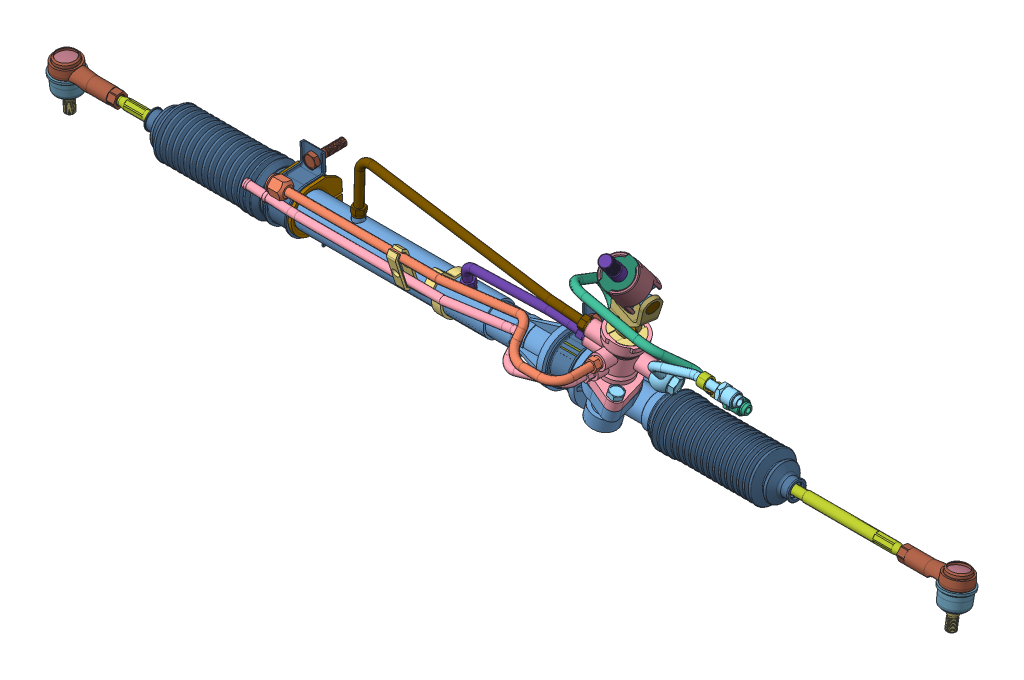
SolidWorks assembly 05, configuration Varsayılan. Lengths in mm.
Overall size (1248.7 288.74 207.21).
83 component instances, 55 part files, 117 mates.
Components (placement in the parent):
- 04-04-1: 04-04 [Varsayılan] at (-125.6681 -6.1583 231.0307) size (234.82 71.44 100.51)
- 04-02-1: 04-02 [Varsayılan] at (196.8103 -6.1583 231.0307) x (0 -1 0) z (-1 0 0) size (38 38 598)
- 04-03-1: 04-03 [Varsayılan] at (38.6923 -33.646 251.0307) x (0.503331 -0.139932 0.852688) z (-0.821509 0.228473 0.52242) size (25.52 151.51 25.52)
- 04-01-1: 04-01 [Varsayılan] at (50.1654 -6.1583 196.9106) x (0 0 1) z (-1 0 0) size (4.12 38.49 38.49)
- 04-05-1: 04-05 [Varsayılan] at (50.1654 -6.1583 220.9669) x (0 0 1) z (-1 0 0) size (15.7 26.77 26.77)
- 04-06-1: 04-06 [Varsayılan] at (50.1654 -6.1583 203.9669) x (-1 0 0) z (0 0 -1) size (18.46 18.46 19.47)
- 04-07-1: 04-07 [Varsayılan] at (50.1654 -6.1583 223.256) x (0 0 1) z (-1 0 0) size (13.68 21.45 8.13)
- 04-08-1: 04-08 [Varsayılan] at (50.1654 -6.1583 218.4607) x (0 1 0) z (-1 0 0) size (28.57 26.12 28.57)
- 05-14-1: 05-14 [Varsayılan] at (37.0194 -39.6612 251.0307) x (0.963448 -0.267897 0) z (0 0 1) size (30.59 16.59 30.59)
- 05-15-1: 05-15 [Varsayılan] at (41.4642 -23.6793 251.0307) x (0.963434 -0.267944 0) z (0 0 1) size (27.84 7.6 27.84)
- 05-21-1: 05-21 [Varsayılan] at (38.6909 -33.6508 251.0307) x (0.928206 -0.258147 -0.267944) z (0.267944 0.963434 0) size (19.84 10.08 10.35)
- 05-09-1: 05-09 [Varsayılan] at (52.7201 16.7933 251.0307) x (0.963434 -0.267944 0) z (0 0 1) size (31.93 8.54 31.93)
- 05-24-1: 05-24 [Varsayılan] at (55.0081 25.0201 251.0307) x (0.963434 -0.267944 0) z (0 0 1) size (34.48 1.46 34.48)
- 05-19-1: 05-19 [Varsayılan] at (66.8414 67.5686 251.0307) x (0.963434 -0.267944 0) z (0 0 1) size (24.62 1.21 24.62)
- 05-10-1: 05-10 [Varsayılan] at (57.7931 35.034 251.0307) x (0.959223 -0.266824 -0.093253) z (0.089843 -0.024987 0.995642) size (34.48 33.93 34.48)
- 05-11-1: 05-11 [Varsayılan] at (60.4905 44.7328 251.0307) x (0.963421 -0.267991 0) z (0 0 1) size (34.47 2.04 34.47)
- 05-11-2: 05-11 [Varsayılan] at (62.3958 51.5836 251.0307) x (0.963421 -0.267991 0) z (0 0 1) size (34.47 2.04 34.47)
- 05-11-3: 05-11 [Varsayılan] at (64.317 58.4915 251.0307) x (0.963421 -0.267991 0) z (0 0 1) size (34.47 2.04 34.47)
- 05-11-4: 05-11 [Varsayılan] at (66.1261 64.9964 251.0307) x (0.963421 -0.267991 0) z (0 0 1) size (34.47 2.04 34.47)
- 05-12-1: 05-12 [Varsayılan] at (67.6164 70.355 251.0307) x (0.92973 -0.25852 0.26224) z (-0.252651 0.070266 0.965003) size (31.17 6.94 31.17)
- 05-13-1: 05-13 [Varsayılan] at (69.4753 77.039 251.0307) x (0.963448 -0.267897 0) z (0 0 1) size (29.11 4.72 29.11)
- 05-16-1: 05-16 [Varsayılan] at (67.6164 70.3552 251.0307) x (0.963448 -0.267897 0) z (0 0 1) size (40.01 14.09 40.01)
- 05-22-3: 05-22 [Varsayılan] at (69.4711 77.024 251.0307) x (0.963434 -0.267944 0) z (0 0 1) size (37.74 2.78 37.74)
- 05-18-1: 05-18 [Varsayılan] at (71.3908 83.9266 251.0307) x (0.96127 -0.267342 0.066993) z (-0.064543 0.01795 0.997753) size (40.8 2.9 40.8)
- 05-25-1: 05-25 [Varsayılan] at (57.2884 33.5525 251.0071) x (0.003637 -0.001047 -0.999993) z (0.963428 -0.267942 0.003784) size (68.03 67.23 77.18)
- formed hex screw_am-1: formed hex screw_am [B18.2.3.2M - Formed hex screw, M10 x 1.5 x 25 --25WS] at (82.3436 33.466 275.1353) x (-0.267944 -0.963434 0) z (0 0 1) size (31.63 18.48 16)
- formed hex screw_am-2: formed hex screw_am [B18.2.3.2M - Formed hex screw, M10 x 1.5 x 25 --25WS] at (36.0727 46.3346 226.9262) x (-0.267944 -0.963434 0) z (0 0 1) size (31.63 18.48 16)
- ROT MİLİ-1: ROT MİLİ [Varsayılan] at (-410.9511 77.9473 255.0381) x (1 0 0) z (0 0.086009 -0.996294) size (284.47 41.76 37.89)
  - 02-02-2: 02-02 [Varsayılan] at (3.7615 85.8588 16.6847) size (48.52 36 36)
  - 02-03-3: 02-03 [Varsayılan] at (0.4735 85.8588 16.6847) x (-1 0 0) z (0 0.000479 1) size (257.66 24 24)
  - 02-01-2: 02-01 [Varsayılan] at (2.815 90.0301 15.9062) x (0.295289 -0.871295 0.391981) z (-0.068342 0.389963 0.918291) size (28 21.64 28)
- ROT MİLİ-2: ROT MİLİ [Varsayılan] at (206.5718 -67.283 293.5918) x (-1 0 0) z (0 -0.568825 -0.822459) size (284.47 41.76 37.89)
  - 02-02-2: 02-02 [Varsayılan] at (3.7615 85.8588 16.6847) size (48.52 36 36)
  - 02-03-3: 02-03 [Varsayılan] at (0.4735 85.8588 16.6847) x (-1 0 0) z (0 0.000479 1) size (257.66 24 24)
  - 02-01-2: 02-01 [Varsayılan] at (2.815 90.0301 15.9062) x (0.295289 -0.871295 0.391981) z (-0.068342 0.389963 0.918291) size (28 21.64 28)
- 05-31-1: 05-31 [Varsayılan] at (-390.0863 -6.1583 231.0307) x (0 0.999978 0.006566) z (0 0.006566 -0.999978) size (59.07 38.45 68.81)
- 05-02-1: 05-02 [Varsayılan] at (-409.0863 -6.1583 231.0307) x (-1 0 0) z (0 -0.999688 0.024965) size (174.75 66.11 66.11)
- 05-02-2: 05-02 [Varsayılan] at (105.6183 -6.1583 231.0307) size (174.75 66.11 66.11)
- ROT BAŞI-1: ROT BAŞI [Varsayılan] at (-661.705 -10.787 321.1728) x (1 0 0) z (0 0.078367 -0.996925) size (99.29 68.51 54.56)
  - 03-01-1: 03-01 [Default] at (-37.7726 9.1069 90.2276) size (90.23 26.88 54.56)
  - 03-02-1: 03-02 [Varsayılan] at (-32.6694 53.6205 89.5242) x (0 -1 0) z (0.136534 0 0.990635) size (58.89 20 20)
  - 03-03-1: 03-03 [Varsayılan] at (-37.7726 -12.3176 90.2276) x (0.135044 0.003215 -0.990834) z (0.99084 0 0.135044) size (26.35 4.4 26.35)
  - 03-04-1: 03-04 [Varsayılan] at (-37.7726 28.686 90.2276) x (0.880691 0 -0.473691) z (0.473691 0 0.880691) size (39.96 25.57 39.96)
  - 03-05-1: 03-05 [Varsayılan] at (-37.7726 -9.866 90.2276) size (25.83 14.98 25.83)
- ROT BAŞI-2: ROT BAŞI [Varsayılan] at (457.3257 -18.6564 141.6394) x (-1 0 0) z (0 0.1653 0.986243) size (99.29 68.51 54.56)
  - 03-01-1: 03-01 [Default] at (-37.7726 9.1069 90.2276) size (90.23 26.88 54.56)
  - 03-02-1: 03-02 [Varsayılan] at (-32.6694 53.6205 89.5242) x (0 -1 0) z (0.136534 0 0.990635) size (58.89 20 20)
  - 03-03-1: 03-03 [Varsayılan] at (-37.7726 -12.3176 90.2276) x (0.135044 0.003215 -0.990834) z (0.99084 0 0.135044) size (26.35 4.4 26.35)
  - 03-04-1: 03-04 [Varsayılan] at (-37.7726 28.686 90.2276) x (0.880691 0 -0.473691) z (0.473691 0 0.880691) size (39.96 25.57 39.96)
  - 03-05-1: 03-05 [Varsayılan] at (-37.7726 -9.866 90.2276) size (25.83 14.98 25.83)
- 05-28-1: 05-28 [Varsayılan] at (-1.0263 -6.1583 231.0307) x (0 -0.759317 -0.650721) z (-1 0 0) size (54.92 54.94 38.56)
- 05-05-3: 05-05 [Varsayılan] at (-153.627 16.7021 236.5228) x (-0.999618 0.007048 -0.026719) z (0.027616 0.221471 -0.974776) size (188.63 111.65 20.5)
- 05-06-2: 05-06 [Varsayılan] at (-308.371 55.2453 229.576) x (-0.999565 0.002273 -0.029406) z (0.029339 -0.025305 -0.999249) size (348.36 140.05 41.18)
- 05-03-3: 05-03 [Varsayılan] at (-414.0863 -6.1583 231.0307) size (295 48.35 43.5)
- 05-33-1: 05-33 [Default] at (-156.8797 44.8002 297.1129) x (-1 0 0) z (0 0.302472 -0.953158) size (421.56 52.06 61.28)
- 05-01-1: 05-01 [Varsayılan] at (-173.5526 -6.1583 231.0307) x (-1 0 0) z (0 0.360562 -0.932735) size (14 137.7 76.92)
- 05-04-1: 05-04 [Varsayılan] at (-390.9146 51.2479 300.523) x (-0.991921 0.112405 0.058801) z (0.000453 0.46666 -0.884437) size (456.96 84.72 60.32)
- 05-08-1: 05-08 [Varsayılan] at (237.637 92.2948 265.4276) x (-0.997325 0.072053 -0.012308) z (-0.043043 -0.714977 -0.697822) size (140.05 46.48 89.04)
- 05-07-1: 05-07 [Varsayılan] at (228.5019 70.3353 246.6946) x (-0.999175 0.040461 0.003581) z (-0.026401 -0.579908 -0.814254) size (231 45.96 100.61)
- formed hex screw_am-3: formed hex screw_am [B18.2.3.2M - Formed hex screw, M12 x 1.75 x 25 --25WS] at (123.6594 37.5337 232.8376) x (-0.948079 0.263674 0.177825) z (-0.177825 -0.903067 0.390959) size (32.76 20.78 18)
- 05-27-1: 05-27 [Varsayılan] at (186.4406 76.9952 250.3773) x (0.044464 0.751851 0.657832) z (0.9987 -0.049876 -0.0105) size (45.68 8 10)
- 05-27-2: 05-27 [Varsayılan] at (196.4276 76.4964 250.2723) x (0.044464 0.751851 0.657832) z (-0.9987 0.049876 0.0105) size (45.68 8 10)
- hex screw_am-2: hex screw_am [B18.6.7M - M5 x 0.8 x 10 Indented HHMS --10S] at (191.9929 87.5632 252.0852) x (-0.024915 -0.657444 0.753091) z (-0.753091 0.507767 0.418362) size (13.8 9.24 8)
- prevailing torque hex nut_am-2: prevailing torque hex nut_am [AM-M5-S] at (191.6665 78.9507 261.9507) x (0.999646 -0.009344 0.024915) z (-0.024915 -0.657444 0.753091) size (8 9.24 5.3)
- 05-29-1: 05-29 [Default] at (-12.3188 -6.1583 205.6444) x (0 1 0) z (0 0 -1) size (108.96 30.28 55.85)
- 05-29-3: 05-29 [Default] at (-390.1285 -6.1115 206.1523) x (0 0.999914 0.013132) z (0 0.013132 -0.999914) size (108.96 30.28 55.85)
- 05-32-2: 05-32 [B18.2.3.2M - Formed hex screw, M10 x 1.5 x 40 --26WS] at (-390.1268 33.0747 215.2976) x (0 0.013132 -0.999914) z (0.935126 0.354284 0.004653) size (46.63 18.48 16)
- 05-32-3: 05-32 [B18.2.3.2M - Formed hex screw, M10 x 1.5 x 40 --26WS] at (-390.1268 -45.812 214.2616) x (0 0.013132 -0.999914) z (0.970956 -0.239236 -0.003142) size (46.63 18.48 16)
- 05-32-4: 05-32 [B18.2.3.2M - Formed hex screw, M10 x 1.5 x 40 --26WS] at (-12.3171 -45.7489 214.2744) x (0 0 -1) z (0.991782 -0.12794 0) size (46.63 18.48 16)
- 05-32-5: 05-32 [B18.2.3.2M - Formed hex screw, M10 x 1.5 x 40 --26WS] at (-12.3171 33.1445 213.7744) x (0 0 -1) z (0.999706 0.024251 0) size (46.63 18.48 16)
- UNIVERSAL MAFSAL-1: UNIVERSAL MAFSAL [Varsayılan] at (141.1705 165.1329 255.0986) x (0.954818 -0.265548 0.133442) z (-0.267944 -0.963434 0) size (48.16 92.97 129.43)
  - 01-01-1: 01-01 [Varsayılan] at (-45.6055 2.036 86.4549) size (47 34.99 57.64)
  - 01-02-1: 01-02 [Varsayılan] at (-45.0363 8.2494 31.8587) x (-0.051046 -0.624854 0.779071) z (0 -0.780088 -0.62567) size (70.3 43.23 43.34)
  - 01-03-1: 01-03 [Varsayılan] at (-51.6055 -0.2661 32.8861) x (1 0 0) z (0 -0.62567 0.780088) size (36 31 16)
  - 01-04-1: 01-04 [Varsayılan] at (-42.5986 38.09 -5.3467) x (-0.998696 0.031938 -0.03982) z (-0.051046 -0.624854 0.779071) size (33.8 41.3 6)
  - 01-05-1: 01-05 [Varsayılan] at (-42.9049 34.3409 -0.6723) x (0.998255 -0.008733 0.058403) z (0.02969 -0.780692 -0.62421) size (32.2 29.4 32.2)
  - 01-06-1: 01-06 [Varsayılan] at (-44.4056 15.9701 22.2324) x (0.051046 0.624854 -0.779071) z (0.993628 0.046715 0.102572) size (75.7 17.29 17.32)
  - 01-07-1: 01-07 [Varsayılan] at (-25.3055 1.2861 40.5406) x (0 0 -1) z (1 0 0) size (16 16 15)
  - 01-08-1: 01-08 [Varsayılan] at (-45.6055 -12.5995 29.4036) x (0.792707 0.38141 -0.475544) z (0 -0.780088 -0.62567) size (16 16 15)
  - 01-07-2: 01-07 [Varsayılan] at (-65.9055 1.2861 40.5406) x (0 -0.633294 0.773912) z (-1 0 0) size (16 16 15)
  - 01-08-2: 01-08 [Varsayılan] at (-45.6055 15.1716 51.6775) x (0.990366 0.086641 -0.108024) z (0 0.780088 0.62567) size (16 16 15)
  - formed hex screw_am-1: formed hex screw_am [B18.2.3.2M - Formed hex screw, M6 x 1.0 x 35 --18WS] at (-62.5055 12.536 76.9549) x (1 0 0) z (0 0.052048 -0.998645) size (39.15 11.55 10)
  - prevailing torque hex nut_am-1: prevailing torque hex nut_am [AM-M6-S] at (-26.1555 12.536 76.9549) x (0 0.889289 0.457347) z (1 0 0) size (10.79 11.55 6.7)
Mates (geometry in assembly coordinates):
- Eş Merkezli1: concentric aligned: cylinder of 04-04-1 through (-165.266 -6.1583 231.0307) axis (1 0 0) radius 14; cylinder of 04-02-1 through (-401.1897 -6.1583 231.0307) axis (1 0 0) radius 11.5
- Eş Merkezli2: concentric anti-aligned: cylinder of 04-04-1 through (54.1024 21.7633 251.0307) axis (0.267944 0.963434 0) radius 12.4576; line of 04-03-1 through (79.2895 112.3276 251.0307) axis (-0.267944 -0.963434 0)
- Teğet1: tangent aligned: plane of 04-04-1 through (55.5026 -19.6951 251.0307) normal (-0.267944 -0.963434 0); cone of 04-03-1 through (43.5006 -16.357 251.0307) axis (-0.267944 -0.963434 0)
- Paralel1: parallel: plane of 04-02-1 through (33.8834 10.9835 238.0307) normal (0 0 1); line of 04-03-1 through (79.2895 112.3276 251.0307) axis (-0.267944 -0.963434 0)
- RackPinionMate1: rack pinion = 20 mm: line of 04-02-1 through (-6.8954 -15.2825 238.0307) axis (-1 0 0); circle of 04-03-1
- Uzaklığı Sınırla1: limit distance = 59.5855 mm anti-aligned: plane of 04-04-1 through (-125.6681 11.3406 231.0307) normal (-1 0 0); plane of 04-02-1 through (-183.1897 -6.1583 250.0307) normal (1 0 0)
- Eş Merkezli3: concentric anti-aligned: cylinder of 04-05-1 through (50.1654 -6.1583 220.9669) axis (0 0 -1) radius 3.705; cylinder of 04-07-1 through (50.1654 -6.1583 223.256) axis (0 0 1) radius 3.7071
- Eş Merkezli4: concentric: sphere of 04-05-1; sphere of 04-07-1
- Eş Merkezli5: concentric anti-aligned: circle of 04-06-1; cylinder of 04-07-1 through (50.1654 -6.1583 223.256) axis (0 0 1) radius 3.7071
- Çakışık1: coincident anti-aligned: plane of 04-05-1 through (59.8031 -6.1583 220.9669) normal (0 0 -1); plane of 04-06-1 through (40.4527 -15.387 220.9669) normal (0 0 1)
- Eş Merkezli6: concentric anti-aligned: circle of 04-06-1; cylinder of 04-08-1 through (50.1654 -6.1583 199.3607) axis (0 0 1) radius 14.285
- Çakışık2: coincident anti-aligned: plane of 04-05-1 through (63.3694 -6.1583 218.4607) normal (0 0 -1); plane of 04-08-1 through (50.1654 -6.1583 218.4607) normal (0 0 1)
- Eş Merkezli7: concentric anti-aligned: cylinder of 04-04-1 through (50.1654 -6.1583 285.0814) axis (0 0 -1) radius 14; cylinder of 04-08-1 through (50.1654 -6.1583 199.3607) axis (0 0 1) radius 14.285
- Çakışık3: coincident anti-aligned: plane of 04-04-1 through (50.1654 -6.1583 201.0307) normal (0 0 -1); circle of 04-08-1
- Eş Merkezli8: concentric anti-aligned: cylinder of 04-04-1 through (50.1654 -6.1583 201.0307) axis (0 0 1) radius 18.85; cylinder of 04-01-1 through (50.1654 -6.1583 196.9106) axis (0 0 -1) radius 13.3852
- Çakışık4: coincident anti-aligned: plane of 04-04-1 through (50.1654 -6.1583 201.0307) normal (0 0 -1); plane of 04-01-1 through (63.5506 -6.1583 201.0307) normal (0 0 1)
- Eş Merkezli9: concentric anti-aligned: cylinder of 04-04-1 through (54.1024 21.7633 251.0307) axis (0.267944 0.963434 0) radius 15.0252; cylinder of 05-15-1 through (43.5005 -16.3572 251.0307) axis (-0.267944 -0.963434 0) radius 13.92
- Çakışık5: coincident anti-aligned: plane of 04-04-1 through (55.5026 -19.6951 251.0307) normal (-0.267944 -0.963434 0); plane of 05-15-1 through (43.5005 -16.3572 251.0307) normal (0.267944 0.963434 0)
- Eş Merkezli10: concentric aligned: cone of 04-03-1 through (38.6923 -33.6458 251.0307) axis (0.267944 0.963434 0); cylinder of 05-21-1 through (38.6909 -33.6508 251.0307) axis (0.267944 0.963434 0) radius 4.26
- Çakışık6: coincident anti-aligned: plane of 05-15-1 through (41.4642 -23.6793 251.0307) normal (-0.267944 -0.963434 0); plane of 05-21-1 through (41.4642 -23.6793 251.0307) normal (0.267944 0.963434 0)
- Eş Merkezli11: concentric aligned: cylinder of 04-04-1 through (54.1024 21.7633 251.0307) axis (0.267944 0.963434 0) radius 15.0252; cone of 05-14-1 through (39.1828 -31.8821 251.0307) axis (0.267944 0.963434 0)
- Teğet2: tangent aligned: cone of 05-14-1 through (41.4644 -23.6786 251.0307) axis (-0.267944 -0.963434 0); plane of 05-15-1 through (41.4642 -23.6793 251.0307) normal (-0.267944 -0.963434 0)
- Çakışık7: coincident: circle of 04-03-1; cone of 05-09-1 through (52.7203 16.7939 251.0307) axis (-0.267944 -0.963434 0)
- Eş Merkezli13: concentric anti-aligned: cylinder of 04-03-1 through (38.6923 -33.646 251.0307) axis (-0.267944 -0.963434 0) radius 12.7592; cone of 05-24-1 through (55.3985 26.4236 251.0307) axis (0.267944 0.963434 0)
- Çakışık8: coincident aligned: cone of 05-09-1 through (55.0081 25.0199 251.0307) axis (-0.267944 -0.963434 0); cone of 05-24-1 through (55.0081 25.0201 251.0307) axis (-0.267944 -0.963434 0)
- Eş Merkezli14: concentric anti-aligned: cone of 04-03-1 through (67.1664 68.7371 251.0307) axis (0.267944 0.963434 0); circle of 05-19-1
- Teğet4: tangent aligned: cone of 04-03-1 through (66.8416 67.5691 251.0307) axis (-0.267944 -0.963434 0); plane of 05-19-1 through (66.8414 67.5686 251.0307) normal (-0.267944 -0.963434 0)
- Eş Merkezli15: concentric anti-aligned: cone of 04-03-1 through (67.1664 68.7371 251.0307) axis (0.267944 0.963434 0); cone of 05-10-1 through (58.0415 35.927 251.0307) axis (-0.267944 -0.963434 0)
- Teğet5: tangent aligned: plane of 05-19-1 through (66.8414 67.5686 251.0307) normal (-0.267944 -0.963434 0); cone of 05-10-1 through (66.8416 67.5691 251.0307) axis (-0.267944 -0.963434 0)
- Eş Merkezli17: concentric aligned: cone of 05-10-1 through (60.4905 44.7328 251.0307) axis (0.267944 0.963434 0); cone of 05-11-1 through (61.036 46.6944 251.0307) axis (0.267944 0.963434 0)
- Çakışık10: coincident: circle of 05-10-1; cone of 05-11-1 through (60.4905 44.7328 251.0307) axis (-0.267944 -0.963434 0)
- Eş Merkezli18: concentric aligned: cone of 05-10-1 through (62.3958 51.5836 251.0307) axis (0.267944 0.963434 0); cone of 05-11-2 through (62.9414 53.5453 251.0307) axis (0.267944 0.963434 0)
- Çakışık11: coincident: circle of 05-10-1; cone of 05-11-2 through (62.3958 51.5836 251.0307) axis (-0.267944 -0.963434 0)
- Eş Merkezli19: concentric aligned: cone of 05-10-1 through (64.317 58.4915 251.0307) axis (0.267944 0.963434 0); cone of 05-11-3 through (64.8625 60.4532 251.0307) axis (0.267944 0.963434 0)
- Çakışık12: coincident: circle of 05-10-1; cone of 05-11-3 through (64.317 58.4915 251.0307) axis (-0.267944 -0.963434 0)
- Eş Merkezli20: concentric aligned: cone of 05-10-1 through (66.1261 64.9964 251.0307) axis (0.267944 0.963434 0); cone of 05-11-4 through (66.6716 66.958 251.0307) axis (0.267944 0.963434 0)
- Çakışık13: coincident: circle of 05-10-1; cone of 05-11-4 through (66.1261 64.9964 251.0307) axis (-0.267944 -0.963434 0)
- Eş Merkezli22: concentric aligned: cone of 04-03-1 through (67.1664 68.7371 251.0307) axis (0.267944 0.963434 0); cone of 05-12-1 through (69.4753 77.039 251.0307) axis (0.267944 0.963434 0)
- Uzaklık1: distance = 2.73 mm aligned: cone of 05-12-1 through (67.6164 70.355 251.0307) axis (-0.267944 -0.963434 0); cone of 05-10-1 through (66.885 67.7251 251.0307) axis (-0.267944 -0.963434 0)
- Eş Merkezli23: concentric aligned: cone of 04-03-1 through (67.1664 68.7371 251.0307) axis (0.267944 0.963434 0); cone of 05-13-1 through (70.7393 81.584 251.0307) axis (0.267944 0.963434 0)
- Çakışık14: coincident aligned: cone of 05-12-1 through (69.4754 77.0393 251.0307) axis (-0.267944 -0.963434 0); cone of 05-13-1 through (69.4753 77.039 251.0307) axis (-0.267944 -0.963434 0)
- Eş Merkezli24: concentric aligned: cone of 05-12-1 through (67.6164 70.3552 251.0307) axis (0.267944 0.963434 0); cone of 05-16-1 through (67.6165 70.3554 251.0307) axis (0.267944 0.963434 0)
- Çakışık15: coincident aligned: cone of 05-12-1 through (67.6164 70.355 251.0307) axis (-0.267944 -0.963434 0); cone of 05-16-1 through (67.6164 70.3552 251.0307) axis (-0.267944 -0.963434 0)
- Eş Merkezli25: concentric anti-aligned: cone of 05-16-1 through (69.4711 77.024 251.0307) axis (0.267944 0.963434 0); cylinder of 05-22-3 through (70.216 79.7023 251.0307) axis (-0.267944 -0.963434 0) radius 18.87
- Çakışık16: coincident aligned: circle of 05-16-1; plane of 05-22-3 through (69.4711 77.024 251.0307) normal (-0.267944 -0.963434 0)
- Eş Merkezli26: concentric anti-aligned: cone of 04-03-1 through (67.1664 68.7371 251.0307) axis (0.267944 0.963434 0); cylinder of 05-18-1 through (76.455 102.1355 251.0307) axis (-0.267944 -0.963434 0) radius 9.8
- Teğet6: tangent aligned: cone of 05-16-1 through (71.3911 83.9275 251.0307) axis (-0.267944 -0.963434 0); plane of 05-18-1 through (71.3908 83.9266 251.0307) normal (-0.267944 -0.963434 0)
- Eş Merkezli27: concentric aligned: cylinder of 04-04-1 through (47.6487 -91.2848 275.1353) axis (0.267944 0.963434 0) radius 5.0797; cylinder of 05-25-1 through (77.2955 15.3149 275.1353) axis (0.267944 0.963434 0) radius 4.95
- Eş Merkezli28: concentric aligned: cylinder of 04-04-1 through (1.3778 -78.4162 226.9262) axis (0.267944 0.963434 0) radius 4.95; cylinder of 05-25-1 through (31.0246 28.1834 226.9262) axis (0.267944 0.963434 0) radius 5.0797
- Çakışık17: coincident anti-aligned: plane of 04-04-1 through (81.3463 14.1883 251.0307) normal (0.267944 0.963434 0); plane of 05-25-1 through (54.0168 21.789 251.0071) normal (-0.267944 -0.963434 0)
- Eş Merkezli291: concentric aligned: cylinder of 05-25-1 through (77.2955 15.3149 275.1353) axis (0.267944 0.963434 0) radius 4.95; cylinder of formed hex screw_am-1 through (82.3436 33.466 275.1353) axis (0.267944 0.963434 0) radius 5
- Çakışık181: coincident anti-aligned: plane of 05-25-1 through (57.2884 33.5525 251.0071) normal (0.267944 0.963434 0); plane of formed hex screw_am-1 through (89.4669 24.6032 275.1353) normal (-0.267944 -0.963434 0)
- Eş Merkezli301: concentric aligned: cylinder of 05-25-1 through (31.0246 28.1834 226.9262) axis (0.267944 0.963434 0) radius 5.0797; cylinder of formed hex screw_am-2 through (36.0727 46.3346 226.9262) axis (0.267944 0.963434 0) radius 5
- Çakışık191: coincident anti-aligned: plane of 05-25-1 through (57.2884 33.5525 251.0071) normal (0.267944 0.963434 0); plane of formed hex screw_am-2 through (43.196 37.4718 226.9262) normal (-0.267944 -0.963434 0)
- Eş Merkezli32: concentric anti-aligned: cylinder of 04-02-1 through (-401.1897 -6.1583 231.0307) axis (1 0 0) radius 11.5; cylinder of ROT MİLİ-1/02-02-2 through (-407.3432 -6.1583 231.0307) axis (-1 0 0) radius 18
- Çakışık20: coincident anti-aligned: plane of 04-02-1 through (-401.1897 -6.1583 231.0307) normal (-1 0 0); plane of ROT MİLİ-1/02-02-2 through (-401.1897 -6.1583 231.0307) normal (1 0 0)
- Eş Merkezli33: concentric aligned: cylinder of 04-02-1 through (-401.1897 -6.1583 231.0307) axis (1 0 0) radius 11.5; cylinder of ROT MİLİ-2/02-02-2 through (202.9638 -6.1583 231.0307) axis (1 0 0) radius 18
- Çakışık21: coincident anti-aligned: plane of 04-02-1 through (196.8103 -6.1583 231.0307) normal (1 0 0); plane of ROT MİLİ-2/02-02-2 through (196.8103 -6.1583 231.0307) normal (-1 0 0)
- Eş Merkezli36: concentric anti-aligned: cylinder of 04-02-1 through (-401.1897 -6.1583 231.0307) axis (1 0 0) radius 11.5; cylinder of 05-02-2 through (105.6183 -6.1583 231.0307) axis (-1 0 0) radius 11.6806
- Çakışık23: coincident anti-aligned: plane of 04-04-1 through (105.6183 12.6764 231.0307) normal (1 0 0); plane of 05-02-2 through (105.6183 19.7754 231.0307) normal (-1 0 0)
- Eş Merkezli37: concentric aligned: cylinder of ROT MİLİ-1/02-03-3 through (-421.4776 -6.1583 231.0307) axis (1 0 0) radius 5.0675; cylinder of ROT BAŞI-1/03-01-1 through (-664.2276 -6.1583 231.0307) axis (1 0 0) radius 9.5
- Çakışık24: coincident aligned: circle of ROT MİLİ-1/02-03-3; plane of ROT BAŞI-1/03-01-1 through (-627.4776 3.069 222.1124) normal (1 0 0)
- Eş Merkezli38: concentric aligned: cylinder of ROT MİLİ-2/02-03-3 through (217.0983 -6.1583 231.0307) axis (-1 0 0) radius 6.5; cylinder of ROT BAŞI-2/03-01-1 through (459.8483 -6.1579 231.0307) axis (-1 0 0) radius 9.5
- Çakışık25: coincident aligned: circle of ROT MİLİ-2/02-03-3; plane of ROT BAŞI-2/03-01-1 through (423.0983 3.8144 239.1074) normal (-1 0 0)
- Eş Merkezli39: concentric anti-aligned: cylinder of 04-04-1 through (-125.6681 -6.1583 231.0307) axis (-1 0 0) radius 21.75; cylinder of 05-28-1 through (-23.5863 -6.1583 231.0307) axis (1 0 0) radius 25.75
- Çakışık26: coincident anti-aligned: plane of 04-04-1 through (6.9737 26.3417 231.0307) normal (-1 0 0); plane of 05-28-1 through (6.9737 -6.1583 231.0307) normal (1 0 0)
- Eş Merkezli304: concentric anti-aligned: cylinder of 05-25-1 through (101.3768 36.6462 241.4658) axis (-0.949417 0.264046 0.169963) radius 5; cylinder of 05-05-3 through (21.6687 58.8141 255.7351) axis (0.949417 -0.264046 -0.169963) radius 7
- Çakışık194: coincident anti-aligned: plane of 05-25-1 through (21.5918 48.3269 253.9468) normal (-0.949417 0.264046 0.169963); plane of 05-05-3 through (26.0012 62.678 256.2827) normal (0.949417 -0.264046 -0.169963)
- Eş Merkezli305: concentric anti-aligned: cylinder of 05-25-1 through (105.7565 50.9201 243.7559) axis (-0.949417 0.264046 0.169963) radius 5; cylinder of 05-06-2 through (26.0484 73.088 258.0251) axis (0.949417 -0.264046 -0.169963) radius 7
- Çakışık195: coincident anti-aligned: plane of 05-25-1 through (21.5918 48.3269 253.9468) normal (-0.949417 0.264046 0.169963); plane of 05-06-2 through (30.1982 77.1184 257.2936) normal (0.949417 -0.264046 -0.169963)
- Eş Merkezli306: concentric anti-aligned: cylinder of 04-02-1 through (-401.1897 -6.1583 231.0307) axis (1 0 0) radius 11.5; cylinder of 05-03-3 through (-119.0863 -6.1583 231.0307) axis (-1 0 0) radius 21.75
- Çakışık196: coincident anti-aligned: plane of 04-04-1 through (-119.0863 12.8417 231.0307) normal (-1 0 0); plane of 05-03-3 through (-119.0863 -6.1583 231.0307) normal (1 0 0)
- Eş Merkezli307: concentric anti-aligned: cylinder of 05-31-1 through (-405.0863 -6.1583 231.0307) axis (1 0 0) radius 20.7084; cylinder of 05-03-3 through (-119.0863 -6.1583 231.0307) axis (-1 0 0) radius 21.75
- Eş Merkezli308: concentric anti-aligned: cylinder of 05-02-1 through (-409.0863 -6.1583 231.0307) axis (1 0 0) radius 25.6827; cylinder of 05-03-3 through (-119.0863 -6.1583 231.0307) axis (-1 0 0) radius 21.75
- Uzaklık2: distance = 5 mm aligned: plane of 05-03-3 through (-414.0863 -6.1583 231.0307) normal (-1 0 0); plane of 05-31-1 through (-409.0863 -6.1583 231.0307) normal (-1 0 0)
- Çakışık197: coincident anti-aligned: plane of 05-31-1 through (-409.0863 -6.1583 231.0307) normal (-1 0 0); plane of 05-02-1 through (-409.0863 -6.8058 205.105) normal (1 0 0)
- Kilitle1: lock: unknown of 05-05-3; unknown of 05-03-3
- Kilitle2: lock: unknown of 05-06-2; unknown of 05-03-3
- Eş Merkezli309: concentric anti-aligned: cylinder of 05-25-1 through (65.5394 62.2675 263.2963) axis (-0.003655 0.006527 0.999972) radius 5; cylinder of 05-33-1 through (65.3201 62.6591 323.2946) axis (0.003655 -0.006527 -0.999972) radius 4
- Çakışık198: coincident anti-aligned: plane of 05-25-1 through (60.6154 54.5186 283.3295) normal (-0.003655 0.006527 0.999972); plane of 05-33-1 through (65.4663 62.3981 283.2958) normal (0.003655 -0.006527 -0.999972)
- Eş Merkezli310: concentric anti-aligned: cylinder of 05-03-3 through (-119.0863 -6.1583 231.0307) axis (-1 0 0) radius 21.75; cylinder of 05-01-1 through (-185.5526 -6.1583 231.0307) axis (1 0 0) radius 21.7671
- Teğet7: tangent anti-aligned: cylinder of 05-33-1 through (-125.1716 75.9211 306.9887) axis (-1 0 0) radius 5; plane of 05-01-1 through (-172.5526 79.1244 302.774) normal (0 -0.309917 0.950763)
- Eş Merkezli312: concentric anti-aligned: cylinder of 05-25-1 through (55.8376 46.5086 263.3637) axis (-0.003655 0.006527 0.999972) radius 5; circle of 05-04-1
- Çakışık201: coincident anti-aligned: plane of 05-25-1 through (60.6154 54.5186 283.3295) normal (-0.003655 0.006527 0.999972); plane of 05-04-1 through (60.0822 49.1995 283.3622) normal (0.003655 -0.006527 -0.999972)
- Kilitle3: lock: unknown of 05-01-1; unknown of 05-04-1
- Eş Merkezli313: concentric aligned: cylinder of 05-25-1 through (18.9204 66.663 252.4828) axis (0.948079 -0.263674 -0.177825) radius 5; cylinder of 05-08-1 through (83.9328 48.5821 240.2888) axis (0.948079 -0.263674 -0.177825) radius 5
- Çakışık202: coincident anti-aligned: plane of 05-25-1 through (97.3407 44.8532 237.774) normal (0.948079 -0.263674 -0.177825); plane of 05-08-1 through (101.3663 42.9237 262.0976) normal (-0.948079 0.263674 0.177825)
- Eş Merkezli314: concentric anti-aligned: cylinder of 05-25-1 through (91.8203 46.3885 292.2446) axis (-0.66663 0.185399 -0.721963) radius 5; cylinder of 05-07-1 through (28.8333 63.9061 224.0295) axis (0.66663 -0.185399 0.721963) radius 3
- Çakışık203: coincident anti-aligned: plane of 05-25-1 through (40.3095 60.7144 222.006) normal (-0.66663 0.185399 -0.721963); plane of 05-07-1 through (29.8159 63.3842 232.381) normal (0.66663 -0.185399 0.721963)
- Eş Merkezli3151: concentric aligned: cylinder of 05-08-1 through (83.9328 48.5821 240.2888) axis (0.948079 -0.263674 -0.177825) radius 5; cylinder of formed hex screw_am-3 through (123.6594 37.5337 232.8376) axis (0.948079 -0.263674 -0.177825) radius 6
- Çakışık2041: coincident anti-aligned: plane of 05-08-1 through (120.4882 37.9933 258.8874) normal (0.948079 -0.263674 -0.177825); plane of formed hex screw_am-3 through (113.5621 36.0564 224.8326) normal (-0.948079 0.263674 0.177825)
- Eş Merkezli316: concentric anti-aligned: cylinder of 05-08-1 through (180.9639 95.1251 266.0234) axis (0.9987 -0.049876 -0.0105) radius 5; cylinder of 05-27-1 through (197.4805 94.3003 265.8497) axis (-0.9987 0.049876 0.0105) radius 8
- Kilitle4: lock: unknown of 05-07-1; unknown of 05-27-1
- Eş Merkezli320: concentric anti-aligned: cylinder of 05-27-1 through (191.5494 75.8607 265.4902) axis (0.024915 0.657444 -0.753091) radius 2.5; cylinder of 05-27-2 through (192.1473 91.6394 247.416) axis (-0.024915 -0.657444 0.753091) radius 2.5
- Çakışık206: coincident anti-aligned: plane of 05-27-1 through (196.4276 76.4964 250.2723) normal (0.024915 0.657444 -0.753091); plane of 05-27-2 through (186.4406 76.9952 250.3773) normal (-0.024915 -0.657444 0.753091)
- Paralel2: parallel aligned: plane of 05-27-1 through (196.1608 71.9853 246.3253) normal (0.9987 -0.049876 -0.0105); plane of 05-27-2 through (196.1608 71.9853 246.3253) normal (0.9987 -0.049876 -0.0105)
- Eş Merkezli3221: concentric anti-aligned: cylinder of 05-27-2 through (192.1473 91.6394 247.416) axis (-0.024915 -0.657444 0.753091) radius 2.5; cylinder of hex screw_am-2 through (192.6257 104.2623 232.9567) axis (0.024915 0.657444 -0.753091) radius 2.5
- Çakışık2091: coincident anti-aligned: plane of 05-27-2 through (187.1989 90.2901 259.353) normal (0.024915 0.657444 -0.753091); plane of hex screw_am-2 through (193.5418 86.4567 256.2164) normal (-0.024915 -0.657444 0.753091)
- Eş Merkezli3231: concentric anti-aligned: cylinder of 05-27-1 through (191.5494 75.8607 265.4902) axis (0.024915 0.657444 -0.753091) radius 2.5; cylinder of prevailing torque hex nut_am-2 through (192.2903 95.4115 243.0952) axis (-0.024915 -0.657444 0.753091) radius 2.5
- Çakışık2101: coincident anti-aligned: plane of 05-27-1 through (197.0863 87.1616 262.2604) normal (-0.024915 -0.657444 0.753091); plane of prevailing torque hex nut_am-2 through (191.7554 85.9152 260.9959) normal (0.024915 0.657444 -0.753091)
- Eş Merkezli324: concentric anti-aligned: cylinder of 05-28-1 through (-23.5863 -6.1583 231.0307) axis (1 0 0) radius 25.75; circle of 05-29-1
- Paralel3: parallel aligned: plane of 04-08-1 through (50.1654 -6.1583 192.3407) normal (0 0 -1); plane of 05-29-1 through (-34.6242 -64.6442 206.6444) normal (0 0 -1)
- Kilitle5: lock: unknown of 05-28-1; unknown of 05-29-1
- Paralel4: parallel aligned: plane of 05-31-1 through (-371.0863 -17.9763 189.9514) normal (0 0 -1); plane of 05-29-1 through (-34.6242 -64.6442 206.6444) normal (0 0 -1)
- Eş Merkezli3233: concentric anti-aligned: cylinder of 05-31-1 through (-405.0863 -6.4449 231.5364) axis (1 0 0) radius 24.365; circle of 05-29-3
- Paralel6: parallel aligned: plane of 05-31-1 through (-409.0863 5.4203 190.105) normal (0 0.013132 -0.999914); plane of 05-29-3 through (-412.4339 -64.6054 206.3842) normal (0 0.013132 -0.999914)
- Kilitle6: lock: unknown of 05-31-1; unknown of 05-29-3
- Eş Merkezli3234: concentric anti-aligned: circle of 05-29-3; cylinder of 05-32-2 through (-390.1268 33.0747 215.2976) axis (0 -0.013132 0.999914) radius 5
- Uzaklık3: distance = 1 mm aligned: plane of 05-32-2 through (-393.3999 41.7993 208.7816) normal (0 0.013132 -0.999914); plane of 05-29-3 through (-412.4339 -64.6054 206.3842) normal (0 0.013132 -0.999914)
- Eş Merkezli32351: concentric aligned: cylinder of 05-29-3 through (-390.1268 -45.5805 196.6331) axis (0 -0.013132 0.999914) radius 6.75; cylinder of 05-32-3 through (-390.1268 -45.812 214.2616) axis (0 -0.013132 0.999914) radius 5
- Çakışık21041: coincident anti-aligned: plane of 05-29-3 through (-402.1268 -39.2149 207.7177) normal (0 -0.013132 0.999914); plane of 05-32-3 through (-387.9167 -36.7564 207.75) normal (0 0.013132 -0.999914)
- Eş Merkezli3236: concentric anti-aligned: circle of 05-29-1; cylinder of 05-32-4 through (-12.3171 -45.7489 214.2744) axis (0 0 1) radius 5
- Çakışık2105: coincident anti-aligned: plane of 05-29-1 through (-24.3171 -39.2383 207.6444) normal (0 0 1); plane of 05-32-4 through (-11.1352 -36.5872 207.6444) normal (0 0 -1)
- Eş Merkezli3237: concentric anti-aligned: circle of 05-29-1; cylinder of 05-32-5 through (-12.3171 33.1445 213.7744) axis (0 0 1) radius 5
- Uzaklık4: distance = 0.5 mm aligned: plane of 05-29-1 through (-34.6242 -64.6442 206.6444) normal (0 0 -1); plane of 05-32-5 through (-12.5411 42.3794 207.1444) normal (0 0 -1)
- Eş Merkezli3238: concentric aligned: line of 04-03-1 through (79.2895 112.3276 251.0307) axis (-0.267944 -0.963434 0); circle of UNIVERSAL MAFSAL-1/01-01-1
- Çakışık2106: coincident aligned: circle of 04-03-1; plane of UNIVERSAL MAFSAL-1/01-01-1 through (56.8513 118.5681 247.8948) normal (-0.267944 -0.963434 0)
